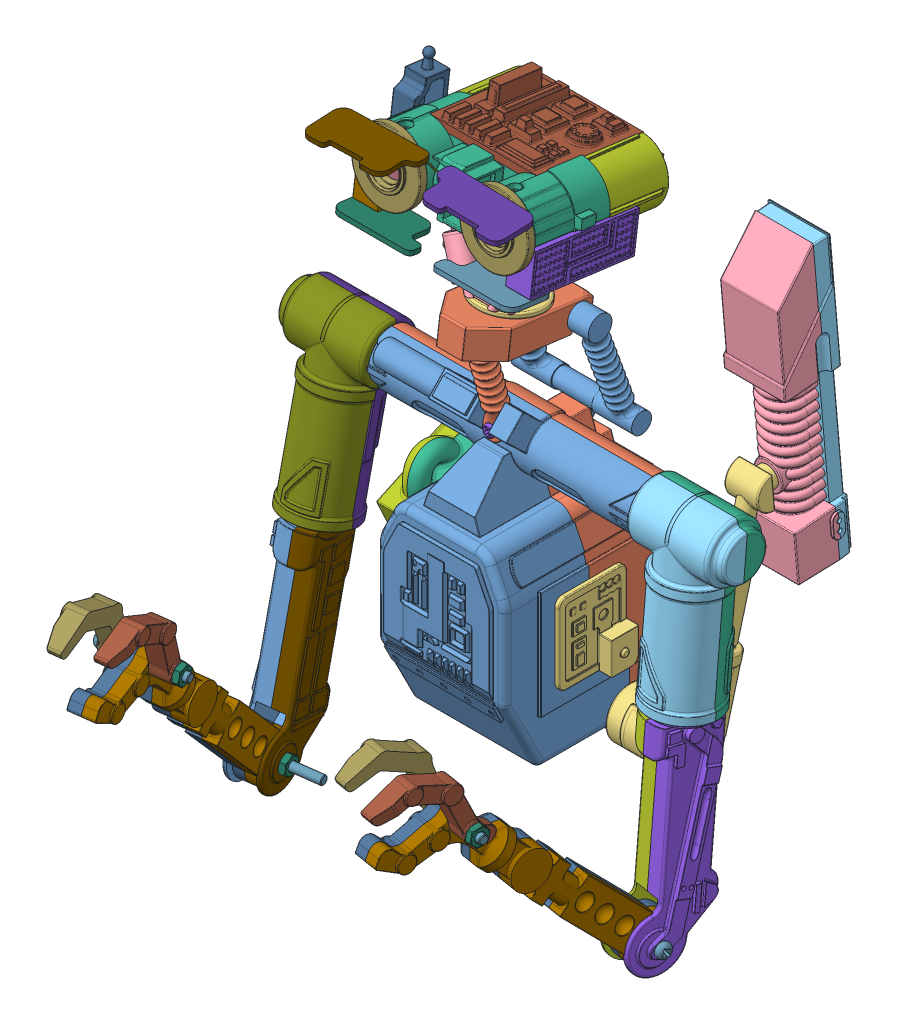
SolidWorks assembly Upper Portion, configuration Painted. Lengths in mm.
Overall size (134.2 209.29 160.81).
74 component instances, 46 part files, 33 mates.
Components (placement in the parent):
- Upper Torso-1: Upper Torso [Painted] at origin size (79.07 88.62 56.86)
  - Upper Torso (Front)-1: Upper Torso (Front) [Default] at origin size (79.07 88.62 40.96)
  - Upper Torso (Rear)-1: Upper Torso (Rear) [Default] at origin size (79.07 84.45 31.52)
  - Upper Torso Detail Plate-1: Upper Torso Detail Plate [Painted] at (20 -40.925 0) x (0 0 -1) z (0 -1 0) size (20.52 5.7 24.35)
  - Cheese Head Thread-Forming Screw 2.8mm x 8mm-1: Cheese Head Thread-Forming Screw 2.8mm x 8mm [Default] at (18 0 3.975) x (1 0 0) z (0 1 0) size (5.45 9.97 5.45)
  - Cheese Head Thread-Forming Screw 2.8mm x 8mm-2: Cheese Head Thread-Forming Screw 2.8mm x 8mm [Default] at (-18 0 3.975) x (1 0 0) z (0 1 0) size (5.45 9.97 5.45)
  - Cheese Head Thread-Forming Screw 2.8mm x 8mm-3: Cheese Head Thread-Forming Screw 2.8mm x 8mm [Default] at (0 -10.15 4.275) x (1 0 0) z (0 1 0) size (5.45 9.97 5.45)
  - Cheese Head Thread-Forming Screw 2.8mm x 8mm-4: Cheese Head Thread-Forming Screw 2.8mm x 8mm [Default] at (10 -64 -9.05) x (1 0 0) z (0 1 0) size (5.45 9.97 5.45)
  - Cheese Head Thread-Forming Screw 2.8mm x 8mm-5: Cheese Head Thread-Forming Screw 2.8mm x 8mm [Default] at (-10 -64 -9.05) x (1 0 0) z (0 1 0) size (5.45 9.97 5.45)
- Arm (Left)-1: Arm (Left) [Default] at (51.85 -26.2988 2.3099) x (1 0 0) z (0 0.087497 0.996165) size (39.72 125.62 97.87)
  - Shoulder (Left, Front)-1: Shoulder (Left, Front) [Default] x (-1 0 0) z (0 0 -1) size (38.1 51.8 11.36)
  - Shoulder (Left, Rear)-1: Shoulder (Left, Rear) [Default] x (-1 0 0) z (0 0 -1) size (38.1 51.8 10.8)
  - Bicep (Left, Inner)-1: Bicep (Left, Inner) [Default] at (0 -14.25 0) x (0.984808 0 0.173648) z (-0.173648 0 0.984808) size (8.6 67 23.2)
  - Bicep (Left, Outer)-1: Bicep (Left, Outer) [Default] at (0 -14.25 0) x (0.984808 0 0.173648) z (-0.173648 0 0.984808) size (8.5 67 23.21)
  - Lower Arm (Left)-1: Lower Arm (Left) [Default] at (-0.9985 -73.25 5.6626) x (0.984808 0 0.173648) z (-0.133022 0.642788 0.754407) size (6.43 23.85 92.58)
  - Lower Arm (Right)-1: Lower Arm (Right) [Default] at (-0.9985 -73.25 5.6626) x (0.984808 0 0.173648) z (-0.133022 0.642788 0.754407) size (6.43 23.85 92.58)
  - Finger (Loutside-Rinside)-1: Finger (Loutside-Rinside) [Default] at (-5.7127 -29.4514 54.2818) x (0.984808 0 0.173648) z (-0.155061 0.45013 0.879397) size (5.9 13.84 36.82)
  - Finger (Linside-Routside)-2: Finger (Linside-Routside) [Default] at (-13.2518 -29.9234 53.2716) x (0.984808 0 0.173648) z (-0.147659 0.526244 0.837415) size (5.9 13.84 36.82)
  - Cheese Head Thread-Forming Screw 2.5mm x 7mm-1: Cheese Head Thread-Forming Screw 2.5mm x 7mm [Default] at (0 10.65 3.4) x (0.707107 -0.707107 0) z (0.707107 0.707107 0) size (4.31 9.04 4.31)
  - Cheese Head Thread-Forming Screw 2.5mm x 7mm-2: Cheese Head Thread-Forming Screw 2.5mm x 7mm [Default] at (0 -11.35 3.4) x (0.707107 -0.707107 0) z (0.707107 0.707107 0) size (4.31 9.04 4.31)
  - Cheese Head Machine Screw 2.5mm x 22mm-1: Cheese Head Machine Screw 2.5mm x 22mm [Default] at (-16.7062 -73.25 2.893) x (0.102255 -0.808233 -0.579917) z (-0.140348 -0.588863 0.795954) size (4.3 24.61 4.3)
  - Cheese Head Machine Screw 2.5mm x 22mm-2: Cheese Head Machine Screw 2.5mm x 22mm [Default] at (2.2832 -26.0878 61.3395) x (-0.015134 0.996195 0.085832) z (-0.172987 -0.087156 0.98106) size (4.3 24.61 4.3)
  - Machine Screw Hex Nut 2.5mm-1: Machine Screw Hex Nut 2.5mm [Default] at (-0.8682 -26.0878 60.7838) x (-0.030154 -0.984808 0.17101) z (-0.17101 0.173648 0.969846) size (5.66 1.9 4.9)
  - Machine Screw Hex Nut 2.5mm-3: Machine Screw Hex Nut 2.5mm [Default] at (-6.5626 -73.25 4.6815) x (0.018381 -0.994382 -0.104246) z (0.172673 0.105854 -0.979275) size (5.66 1.9 4.9)
- Arm (Right)-1: Arm (Right) [Default] at (-51.85 -25.7724 5.7222) x (1 0 0) z (0 0.216749 0.976227) size (40.56 126.04 102.41)
  - Shoulder (Right, Front)-1: Shoulder (Right, Front) [Default] at origin size (38.1 51.8 11.36)
  - Shoulder (Right, Rear)-1: Shoulder (Right, Rear) [Default] at origin size (38.1 51.8 10.8)
  - Bicep (Right, Inner)-1: Bicep (Right, Inner) [Default] at (0 -14.25 0) x (0.984808 0 -0.173648) z (0.173648 0 0.984808) size (8.6 67 23.2)
  - Bicep (Right, Outer)-1: Bicep (Right, Outer) [Default] at (0 -14.25 0) x (0.984808 0 -0.173648) z (0.173648 0 0.984808) size (8.5 67 23.21)
  - Lower Arm (Left)-1: Lower Arm (Left) [Default] at (0.9985 -73.25 5.6626) x (0.984808 0 -0.173648) z (0.142244 0.573576 0.806707) size (6.43 23.85 92.58)
  - Lower Arm (Right)-1: Lower Arm (Right) [Default] at (0.9985 -73.25 5.6626) x (0.984808 0 -0.173648) z (0.142244 0.573576 0.806707) size (6.43 23.85 92.58)
  - Finger (Loutside-Rinside)-1: Finger (Loutside-Rinside) [Default] at (13.8752 -34.3601 56.8067) x (0.984808 0 -0.173648) z (0.155061 0.45013 0.879397) size (5.9 13.84 36.82)
  - Finger (Linside-Routside)-2: Finger (Linside-Routside) [Default] at (6.3434 -33.8625 57.8586) x (0.984808 0 -0.173648) z (0.161284 0.37059 0.914686) size (5.9 13.84 36.82)
  - Cheese Head Thread-Forming Screw 2.5mm x 7mm-1: Cheese Head Thread-Forming Screw 2.5mm x 7mm [Default] at (0 10.65 3.4) x (0.707107 -0.707107 0) z (0.707107 0.707107 0) size (4.31 9.04 4.31)
  - Cheese Head Thread-Forming Screw 2.5mm x 7mm-2: Cheese Head Thread-Forming Screw 2.5mm x 7mm [Default] at (0 -11.35 3.4) x (0.707107 -0.707107 0) z (0.707107 0.707107 0) size (4.31 9.04 4.31)
  - Cheese Head Machine Screw 2.5mm x 22mm-1: Cheese Head Machine Screw 2.5mm x 22mm [Default] at (16.7062 -73.25 2.893) x (-0.102255 -0.808233 -0.579917) z (-0.140348 0.588863 -0.795954) size (4.3 24.61 4.3)
  - Cheese Head Machine Screw 2.5mm x 22mm-2: Cheese Head Machine Screw 2.5mm x 22mm [Default] at (23.8028 -30.9964 60.704) x (0.030154 0.984808 0.17101) z (0.17101 -0.173648 0.969846) size (4.3 24.61 4.3)
  - Machine Screw Hex Nut 2.5mm-1: Machine Screw Hex Nut 2.5mm [Default] at (20.6514 -30.9964 61.2597) x (0.015134 -0.996195 0.085832) z (0.172987 0.087156 0.98106) size (5.66 1.9 4.9)
  - Machine Screw Hex Nut 2.5mm-3: Machine Screw Hex Nut 2.5mm [Default] at (6.5626 -73.25 4.6815) x (-0.15873 -0.405519 -0.9002) z (0.070418 -0.914087 0.399358) size (5.66 1.9 4.9)
- Head-1: Head [Painted] at (0 28.7083 5.1429) x (1 0 0) z (0 0.129856 0.991533) size (59.38 58.47 64.88)
  - Neck Block-1: Neck Block [Default] at origin size (19.8 8.1 32.9)
  - Neck Column-1: Neck Column [Default] at (0 8.1 0) size (19.3 30.7 19.3)
  - Neck Cylinders-1: Neck Cylinders [Default] at (0 9.78 6.15) size (41.82 28.67 7.85)
  - Washer Head Thread-Forming Screw 2.6mm x 6mm-1: Washer Head Thread-Forming Screw 2.6mm x 6mm [Default] at (0 11.65 0) x (-0.707107 0 -0.707107) z (-0.707107 0 0.707107) size (7.8 7.44 7.8)
  - Head (Front)-1: Head (Front) [Default] at (0 40.98 0) size (53.5 23.44 24.2)
  - Head (Rear)-1: Head (Rear) [Default] at (0 40.98 0) size (51.98 22.63 26)
  - Cheese Head Thread-Forming Screw 2.8mm x 8mm-1: Cheese Head Thread-Forming Screw 2.8mm x 8mm [Default] at (0 40.98 3.65) x (0.707107 -0.707107 0) z (0.707107 0.707107 0) size (5.45 9.97 5.45)
  - Cheek (Left)-1: Cheek (Left) [Default] at (16.25 40.98 23) size (7.5 12 31.6)
  - Cheek (Right)-1: Cheek (Right) [Default] at (-16.25 40.98 23) size (7.5 12 31.6)
  - Whip Antenna-1: Whip Antenna [Default] at (-26.586 40.0668 10.4) size (6.56 18.4 10.28)
  - Head Detail Plate-1: Head Detail Plate [Default] at (0 47.98 -2.935) size (32.69 7.75 31.87)
  - Eye-3: Eye [Default] at (-16.25 40.98 23) size (20.5 20.5 7.96)
  - Eye-4: Eye [Default] at (16.25 40.98 23) size (20.5 20.5 7.96)
  - Lens-1: Lens [Painted] at (-16.25 40.98 23) size (10.8 10.8 0.8)
  - Lens-2: Lens [Painted] at (16.25 40.98 23) size (10.8 10.8 0.8)
  - Lower Eyeflap (Left)-1: Lower Eyeflap (Left) [Default] at (3.25 26.4828 29.4) size (23.8 1.32 12.82)
  - Lower Eyeflap (Right)-1: Lower Eyeflap (Right) [Default] at (-3.25 26.4828 29.4) size (23.8 1.32 12.82)
  - Eyeflap Wire-1: Eyeflap Wire [Default] at (0 46.2834 36.3285) x (1 0 0) z (0 0.173648 0.984808) size (22.36 3.31 16.37)
  - Upper Eyeflap (Left)-1: Upper Eyeflap (Left) [Default] at (2.6277 49.0084 30.8173) x (0.99978 -0.019812 0.006846) z (-0.010094 -0.168795 0.985599) size (26.82 1.32 12.82)
  - Upper Eyeflap (Right)-1: Upper Eyeflap (Right) [Default] at (-2.6331 49.0082 30.8174) x (0.999778 0.019901 -0.006876) z (0.010139 -0.168839 0.985592) size (26.82 1.32 12.82)
- Neck Rods (Rear)-1: Neck Rods (Rear) [Default] at (0 2.05 -17.7) size (36.3 40.73 17.15)
- Neck Rod (Front)-1: Neck Rod (Front) [Default] at (0 7.8374 7.2098) x (1 0 0) z (0 -0.261344 0.965246) size (6.66 34 7.11)
- Accessory Mount-1: Accessory Mount [Painted] at (19.25 -69.9 -12.95) x (1 0 0) z (0 0.258819 0.965926) size (25.77 76.05 18.88)
- Laser-1: Laser [Default] at (39.45 -33.0223 -46.791) x (1 0 0) z (0 0.996195 0.087156) size (19.97 16.85 86.4)
  - Laser (Bottom)-1: Laser (Bottom) [Default] at origin size (19.97 12.05 86.4)
  - Laser (Top)-1: Laser (Top) [Default] at origin size (19.97 4.8 86.4)
- Toolbox-1: Toolbox [Painted] at (39.45 -29.2379 -36.1206) x (1 0 0) z (0 0.996195 0.087156) size (32.95 30.38 95) (hidden)
  - Toolbox (Bottom)-1: Toolbox (Bottom) [Default] at origin size (32.95 16.43 95)
  - Toolbox (Top)-1: Toolbox (Top) [Painted] at (0 12.5 0) size (31.39 19.55 95)
- Tool Arm-1: Tool Arm [Default] at (-30.25 -22.9673 -7.9466) x (1 0 0) z (0 0.906308 0.422618) size (19.65 32.1 67.19)
  - Tool Arm (Inner)-1: Tool Arm (Inner) [Default] at origin size (12.5 31.7 67.16)
  - Tool Arm (Outer)-1: Tool Arm (Outer) [Default] at origin size (9.65 32.1 67.19)
- Cheese Head Self-Tapping Screw 2mm x 8mm-2: Cheese Head Self-Tapping Screw 2mm x 8mm [Default] at (0 -3 -10.825) x (0.707107 0.707107 0) z (-0.707107 0.707107 0) size (3.5 9.41 3.5)
- Cheese Head Self-Tapping Screw 2mm x 8mm-3: Cheese Head Self-Tapping Screw 2mm x 8mm [Default] at (0 4.0803 1.0493) x (0.704556 0.707107 -0.060001) z (0.709648 -0.702034 0.059571) size (3.5 9.41 3.5)
Mates (geometry in assembly coordinates):
- Coincident1: coincident: plane of ? through (0 0 0) normal (1 0 0); plane of assembly through (0 0 0) normal (1 0 0)
- Coincident2: coincident: plane of ? through (0 0 0) normal (0 0 1); plane of assembly through (0 0 0) normal (0 0 1)
- Coincident3: coincident aligned: plane of ? through (0 0 0) normal (0 1 0); plane of assembly through (0 0 0) normal (0 1 0)
- Concentric1: concentric aligned: cylinder of ? through (24.95 0 0) axis (1 0 0) radius 5; cylinder of ? through (29 0 0) axis (1 0 0) radius 5.15
- Concentric2: concentric aligned: cylinder of ? through (-24.95 0 0) axis (-1 0 0) radius 5; cylinder of ? through (-29 0 0) axis (-1 0 0) radius 5.15
- Coincident4: coincident anti-aligned: plane of ? through (-39.45 0 0) normal (-1 0 0); circle of ?
- Coincident5: coincident aligned: plane of ? through (39.45 0 0) normal (1 0 0); circle of ?
- Concentric4: concentric anti-aligned: cylinder of ? through (15.25 -69.9 -12.95) axis (1 0 0) radius 5.8; cylinder of Accessory Mount-1 through (35.55 -69.9 -12.95) axis (-1 0 0) radius 5.8
- Concentric5: concentric aligned: cylinder of Accessory Mount-1 through (39.45 -8.9517 -39.666) axis (0 -0.087156 0.996195) radius 3.15; cylinder of ? through (39.45 -8.9517 -39.666) axis (0 -0.087156 0.996195) radius 2.99
- Coincident6: coincident anti-aligned: plane of Accessory Mount-1 through (39.45 -8.9517 -39.666) normal (0 0.087156 -0.996195); plane of ? through (39.45 -8.9517 -39.666) normal (0 -0.087156 0.996195)
- Parallel1: parallel aligned: plane of Accessory Mount-1; plane of ?
- Concentric6: concentric aligned: cylinder of Accessory Mount-1 through (39.45 -8.9517 -39.666) axis (0 -0.087156 0.996195) radius 3.15; cylinder of Toolbox-1/Toolbox (Bottom)-1 through (39.45 -8.9517 -39.666) axis (0 -0.087156 0.996195) radius 2.96
- Coincident8: coincident anti-aligned: plane of Accessory Mount-1 through (39.45 -8.9517 -39.666) normal (0 0.087156 -0.996195); plane of Toolbox-1/Toolbox (Bottom)-1 through (39.45 -8.9517 -39.666) normal (0 -0.087156 0.996195)
- Parallel2: parallel aligned: plane of Accessory Mount-1; plane of Toolbox-1/Toolbox (Bottom)-1
- Angle1: planar angle = 0.261799 rad aligned: plane of Accessory Mount-1 through (19.25 -69.9 -12.95) normal (0 0.258819 0.965926); plane of ? through (0 0 0) normal (0 0 1)
- Coincident9: coincident anti-aligned: plane of ? through (19.25 0 0) normal (1 0 0); plane of Accessory Mount-1 through (19.25 -69.9 -12.95) normal (-1 0 0)
- Concentric7: concentric anti-aligned: cylinder of ? through (0 -3 -16.425) axis (0 0 -1) radius 0.75; cylinder of Neck Rods (Rear)-1 through (0 -3 -20.7) axis (0 0 1) radius 1.25
- Coincident10: coincident anti-aligned: plane of ? through (8.5 -6.8 -16.425) normal (0 0 -1); plane of Neck Rods (Rear)-1 through (0 -3 -16.425) normal (0 0 1)
- Concentric8: concentric aligned: cylinder of Head-1/Neck Block-1 through (-9.9 30.5305 -7.0974) axis (1 0 0) radius 1.5038; cylinder of Neck Rods (Rear)-1 through (-18.15 30.5305 -7.0974) axis (1 0 0) radius 1.4
- Coincident11: coincident aligned: plane of Head-1/Neck Block-1; plane of Neck Rods (Rear)-1 through (0 2.05 -17.7) normal (1 0 0)
- Coincident13: coincident aligned: plane of Neck Rods (Rear)-1 through (0 2.05 -17.7) normal (1 0 0); plane of assembly through (0 0 0) normal (1 0 0)
- Concentric9: concentric aligned: cylinder of ? through (0 4.5433 6.5062) axis (0 0.084551 0.996419) radius 0.75; cylinder of Neck Rod (Front)-1 through (0 4.1798 2.2222) axis (0 0.084551 0.996419) radius 1.25
- Coincident12: coincident aligned: plane of assembly through (0 0 0) normal (1 0 0); plane of Neck Rod (Front)-1
- Concentric10: concentric anti-aligned: cylinder of Neck Rods (Rear)-1 through (0 -3 -20.7) axis (0 0 1) radius 1.25; cylinder of Cheese Head Self-Tapping Screw 2mm x 8mm-2 through (0 -3 -20.235) axis (0 0 -1) radius 1
- Angle3: planar angle = 0.785398 rad aligned: plane of Cheese Head Self-Tapping Screw 2mm x 8mm-2; plane of assembly through (0 0 0) normal (0 1 0)
- Coincident14: coincident anti-aligned: plane of Neck Rods (Rear)-1 through (0 -3 -18.975) normal (0 0 -1); plane of Cheese Head Self-Tapping Screw 2mm x 8mm-2 through (-0.7071 -3.7071 -18.975) normal (0 0 1)
- Angle4: planar angle = 0.785398 rad aligned: plane of Cheese Head Self-Tapping Screw 2mm x 8mm-3; plane of assembly through (0 0 0) normal (0 1 0)
- Concentric11: concentric aligned: cylinder of Neck Rod (Front)-1 through (0 4.1798 2.2222) axis (0 0.084551 0.996419) radius 1.25; cylinder of Cheese Head Self-Tapping Screw 2mm x 8mm-3 through (0 4.8759 10.4256) axis (0 0.084551 0.996419) radius 1
- Tangent2: tangent: face of Neck Rod (Front)-1; plane of Cheese Head Self-Tapping Screw 2mm x 8mm-3 through (-0.7046 4.0622 9.2301) normal (0 -0.084551 -0.996419)
- Coincident15: coincident: point of Head-1/Neck Block-1; point of Neck Rod (Front)-1
- Concentric12: concentric anti-aligned: cylinder of ? through (-15.25 -69.9 -12.95) axis (-1 0 0) radius 5.8; cone of ? through (-19.9 -69.9 -12.95) axis (1 0 0)
- Angle5: planar angle = 0.436332 rad anti-aligned: plane of ? through (-30.25 -22.9673 -7.9466) normal (0 0.422618 -0.906308)
- Distance1: distance = 0.7 mm anti-aligned: plane of ? through (-19.95 -69.9 -12.95) normal (1 0 0); plane of ? through (-19.25 0 0) normal (-1 0 0)
